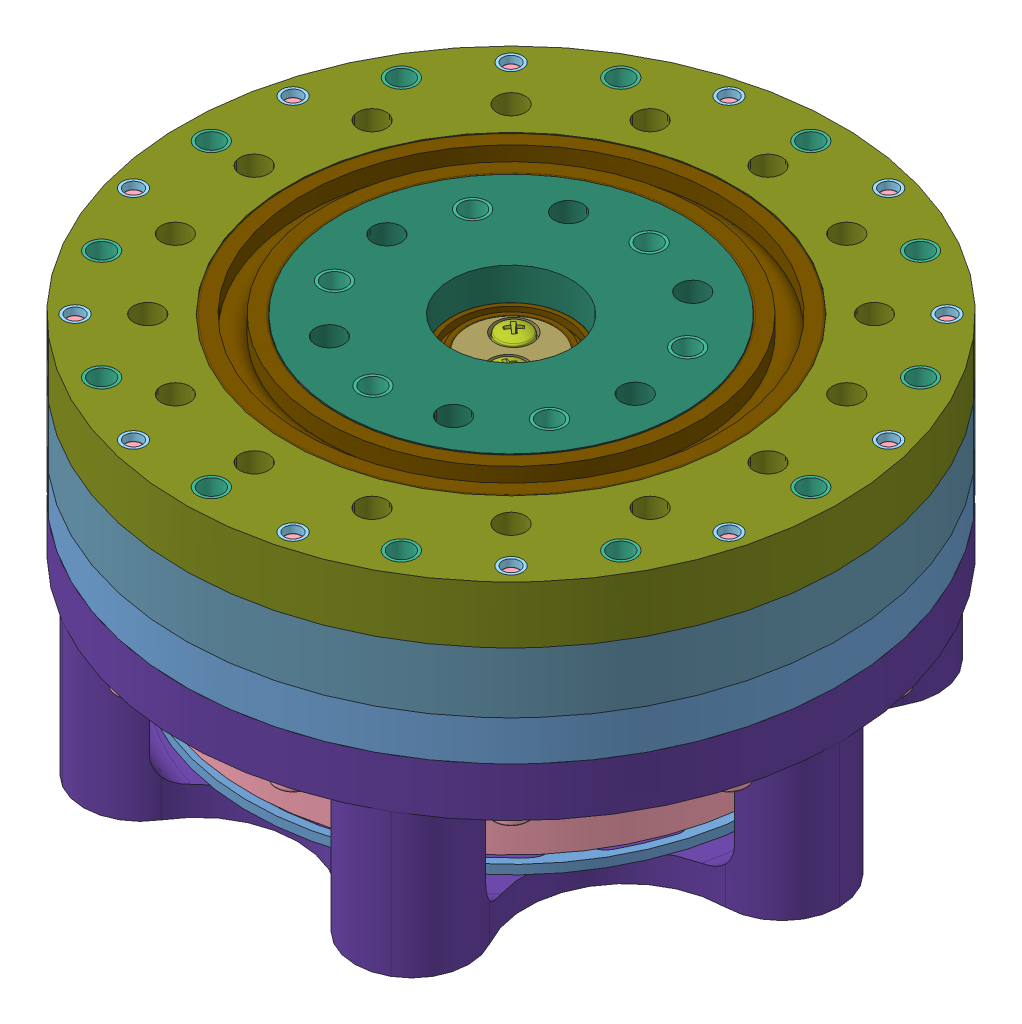
SolidWorks assembly Cycloidal, configuration Default. Lengths in mm.
Overall size (162.63 70.39 162.63).
392 component instances, 94 part files, 246 mates.
Components (placement in the parent):
- motor-X83008S.stp-1: motor-X83008S.stp [Default] at (19.7719 89.7915 55.1095) x (0.817868 0 0.575406) z (0 -1 0) size (114.7 114.7 37.62)
  - base.stp-1: base.stp [Default] at (42.0794 12.0269 46.7342) size (91.6 91.6 15.61)
  - stator.stp-1: stator.stp [Default] at (42.0794 12.0269 33.1342) x (0.08493 -0.996387 0) z (0 0 1) size (83 83 8)
  - coil.stp-1: coil.stp [Default] at (39.5332 41.8984 37.1342) x (0.996387 0.08493 0) z (-0.08493 0.996387 0) size (4.4 10.2 10.5)
  - coil.stp-2: coil.stp [Default] at (34.3848 41.0025 37.1342) x (0.966502 0.256661 0) z (-0.256661 0.966502 0) size (4.4 10.2 10.5)
  - coil.stp-3: coil.stp [Default] at (29.4701 39.2261 37.1342) x (0.90725 0.420593 0) z (-0.420593 0.90725 0) size (4.4 10.2 10.5)
  - coil.stp-4: coil.stp [Default] at (24.9386 36.6233 37.1342) x (0.820431 0.571745 0) z (-0.571745 0.820431 0) size (4.4 10.2 10.5)
  - coil.stp-5: coil.stp [Default] at (20.9279 33.2732 37.1342) x (0.708685 0.705525 0) z (-0.705525 0.708685 0) size (4.4 10.2 10.5)
  - coil.stp-6: coil.stp [Default] at (17.5599 29.2775 37.1342) x (0.575405 0.817869 0) z (-0.817869 0.575405 0) size (4.4 10.2 10.5)
  - coil.stp-7: coil.stp [Default] at (14.9368 24.7576 37.1342) x (0.424642 0.905361 0) z (-0.905361 0.424642 0) size (4.4 10.2 10.5)
  - coil.stp-8: coil.stp [Default] at (13.1385 19.8509 37.1342) x (0.260976 0.965345 0) z (-0.965345 0.260976 0) size (4.4 10.2 10.5)
  - coil.stp-9: coil.stp [Default] at (12.2196 14.7066 37.1342) x (0.089381 0.995998 0) z (-0.995998 0.089381 0) size (4.4 10.2 10.5)
  - coil.stp-10: coil.stp [Default] at (12.2079 9.4807 37.1342) x (-0.08493 0.996387 0) z (-0.996387 -0.08493 0) size (4.4 10.2 10.5)
  - coil.stp-11: coil.stp [Default] at (13.1039 4.3323 37.1342) x (-0.256661 0.966502 0) z (-0.966502 -0.256661 0) size (4.4 10.2 10.5)
  - coil.stp-12: coil.stp [Default] at (14.8802 -0.5824 37.1342) x (-0.420593 0.90725 0) z (-0.90725 -0.420593 0) size (4.4 10.2 10.5)
  - coil.stp-13: coil.stp [Default] at (17.483 -5.1139 37.1342) x (-0.571745 0.820431 0) z (-0.820431 -0.571745 0) size (4.4 10.2 10.5)
  - coil.stp-14: coil.stp [Default] at (20.8332 -9.1246 37.1342) x (-0.705525 0.708685 0) z (-0.708685 -0.705525 0) size (4.4 10.2 10.5)
  - coil.stp-15: coil.stp [Default] at (24.8289 -12.4926 37.1342) x (-0.817869 0.575405 0) z (-0.575405 -0.817869 0) size (4.4 10.2 10.5)
  - coil.stp-16: coil.stp [Default] at (29.3487 -15.1157 37.1342) x (-0.905361 0.424642 0) z (-0.424642 -0.905361 0) size (4.4 10.2 10.5)
  - coil.stp-17: coil.stp [Default] at (34.2554 -16.914 37.1342) x (-0.965345 0.260976 0) z (-0.260976 -0.965345 0) size (4.4 10.2 10.5)
  - coil.stp-18: coil.stp [Default] at (39.3998 -17.8329 37.1342) x (-0.995998 0.089381 0) z (-0.089381 -0.995998 0) size (4.4 10.2 10.5)
  - coil.stp-19: coil.stp [Default] at (44.6256 -17.8446 37.1342) x (-0.996387 -0.08493 0) z (0.08493 -0.996387 0) size (4.4 10.2 10.5)
  - coil.stp-20: coil.stp [Default] at (49.7741 -16.9486 37.1342) x (-0.966502 -0.256661 0) z (0.256661 -0.966502 0) size (4.4 10.2 10.5)
  - coil.stp-21: coil.stp [Default] at (54.6887 -15.1723 37.1342) x (-0.90725 -0.420593 0) z (0.420593 -0.90725 0) size (4.4 10.2 10.5)
  - coil.stp-22: coil.stp [Default] at (59.2202 -12.5695 37.1342) x (-0.820431 -0.571745 0) z (0.571745 -0.820431 0) size (4.4 10.2 10.5)
  - coil.stp-23: coil.stp [Default] at (63.2309 -9.2193 37.1342) x (-0.708685 -0.705525 0) z (0.705525 -0.708685 0) size (4.4 10.2 10.5)
  - coil.stp-24: coil.stp [Default] at (66.599 -5.2236 37.1342) x (-0.575405 -0.817869 0) z (0.817869 -0.575405 0) size (4.4 10.2 10.5)
  - coil.stp-25: coil.stp [Default] at (69.222 -0.7038 37.1342) x (-0.424642 -0.905361 0) z (0.905361 -0.424642 0) size (4.4 10.2 10.5)
  - coil.stp-26: coil.stp [Default] at (71.0203 4.2029 37.1342) x (-0.260976 -0.965345 0) z (0.965345 -0.260976 0) size (4.4 10.2 10.5)
  - coil.stp-27: coil.stp [Default] at (71.9392 9.3473 37.1342) x (-0.089381 -0.995998 0) z (0.995998 -0.089381 0) size (4.4 10.2 10.5)
  - coil.stp-28: coil.stp [Default] at (71.9509 14.5731 37.1342) x (0.08493 -0.996387 0) z (0.996387 0.08493 0) size (4.4 10.2 10.5)
  - coil.stp-29: coil.stp [Default] at (71.055 19.7216 37.1342) x (0.256661 -0.966502 0) z (0.966502 0.256661 0) size (4.4 10.2 10.5)
  - coil.stp-30: coil.stp [Default] at (69.2786 24.6362 37.1342) x (0.420593 -0.90725 0) z (0.90725 0.420593 0) size (4.4 10.2 10.5)
  - coil.stp-31: coil.stp [Default] at (66.6758 29.1677 37.1342) x (0.571745 -0.820431 0) z (0.820431 0.571745 0) size (4.4 10.2 10.5)
  - coil.stp-32: coil.stp [Default] at (63.3257 33.1785 37.1342) x (0.705525 -0.708685 0) z (0.708685 0.705525 0) size (4.4 10.2 10.5)
  - coil.stp-33: coil.stp [Default] at (59.33 36.5465 37.1342) x (0.817869 -0.575405 0) z (0.575405 0.817869 0) size (4.4 10.2 10.5)
  - coil.stp-34: coil.stp [Default] at (54.8101 39.1695 37.1342) x (0.905361 -0.424642 0) z (0.424642 0.905361 0) size (4.4 10.2 10.5)
  - coil.stp-35: coil.stp [Default] at (49.9034 40.9678 37.1342) x (0.965345 -0.260976 0) z (0.260976 0.965345 0) size (4.4 10.2 10.5)
  - coil.stp-36: coil.stp [Default] at (44.759 41.8868 37.1342) x (0.995998 -0.089381 0) z (0.089381 0.995998 0) size (4.4 10.2 10.5)
  - rotor.stp-1: rotor.stp [Default] at (42.0794 12.0269 42.1342) x (-0.293442 0.955977 0) z (0 0 -1) size (91.8 91.8 12)
  - outrunner.stp-1: outrunner.stp [Default] at (42.0794 12.0269 30.1342) x (-0.254711 0.967017 0) z (-0.967017 -0.254711 0) size (91.8 17.01 91.8)
  - screw-mount.stp-1: screw-mount.stp [Default] at (38.1314 27.0157 27.1342) x (1 0 0) z (0 0 -1) size (7 7 6.5)
  - screw-mount.stp-2: screw-mount.stp [Default] at (27.0906 8.0789 27.1342) x (1 0 0) z (0 0 -1) size (7 7 6.5)
  - screw-mount.stp-3: screw-mount.stp [Default] at (57.0682 15.9749 27.1342) x (1 0 0) z (0 0 -1) size (7 7 6.5)
  - screw-mount.stp-4: screw-mount.stp [Default] at (46.0274 -2.9618 27.1342) x (1 0 0) z (0 0 -1) size (7 7 6.5)
  - 6702ZZ-bearing-15x21x4.stp-1: 6702ZZ-bearing-15x21x4.stp [Default] at (42.0794 12.0269 43.7342) x (1 0 0) z (0 -1 0) size (21 4 21)
  - 6702ZZ-bearing-15x21x4.stp-2: 6702ZZ-bearing-15x21x4.stp [Default] at (42.0794 12.0269 35.1342) x (1 0 0) z (0 1 0) size (21 4 21)
  - shaft.stp-1: shaft.stp [Default] at (42.0794 12.0269 20.1342) size (16 16 31.6)
  - fix-screw.stp-1: fix-screw.stp [Default] at (42.0794 12.0269 51.7342) x (1 0 0) z (0 0 -1) size (19.67 18.96 12.02)
- Base_Plate-1: Base_Plate [Default] at (47.267 69.6573 89.1587) x (-0.64433 0 -0.764747) z (0.764747 0 -0.64433) size (40 7 40)
- Eccentric_Shaft-1: Eccentric_Shaft [Default] at (62.181 70.3165 95.0179) x (-0.764747 0 0.64433) z (-0.64433 0 -0.764747) size (20 15 17)
  - Eccentric_Shaft_bot-1: Eccentric_Shaft_bot [Default] at (7.6302 6.3409 14.0904) size (17 5 17)
  - Eccentric_Shaft_bot-2: Eccentric_Shaft_bot [Default] at (7.6302 11.3409 14.0904) x (-1 0 0) z (0 0 -1) size (17 5 17)
  - Eccentric_Shaft_top-1: Eccentric_Shaft_top [Default] at (7.6302 16.3409 14.0904) x (-1 0 0) z (0 0 -1) size (17 5 17)
- Cycloidal_Discs-1: Cycloidal_Discs [Default] at (46.1199 86.6573 90.1252) x (0.999784 0 -0.020763) z (-0.020763 0 -0.999784) size (79.25 5 79.73)
- Cycloidal_Discs-2: Cycloidal_Discs [Default] at (48.4141 76.6573 88.1922) x (0.979859 0 0.19969) z (-0.19969 0 0.979859) size (79.25 5 79.73)
- Ring_Pin_Housing-1: Ring_Pin_Housing [Default] at (47.267 76.6573 89.1587) x (0.707107 0 -0.707107) z (0.707107 0 0.707107) size (115 10.6 115)
- Output_Shaft-1: Output_Shaft [Default] at (47.267 87.2573 89.1587) x (-0.998587 0 -0.053142) z (0.053142 0 -0.998587) size (60 10 60)
- Cover-1: Cover [Default] at (47.267 87.2573 89.1587) x (0.707107 0 -0.707107) z (0.707107 0 0.707107) size (115 10.4 115)
- Motor_Cover-2: Motor_Cover [Default] at (47.267 36.0573 89.1587) size (115 33.6 115)
- radial ball bearing_68_iso-39: radial ball bearing_68_iso [ISO 15 RBB - 1860 - 32,SI,NC,32_68] at (47.267 92.2573 89.1587) x (0 1 0) z (0 0 1) size (10 78 78)
- radial ball bearing_68_iso-40: radial ball bearing_68_iso [ISO 15 RBB - 1840 - 32,SI,NC,32_68] at (47.267 72.9573 89.1587) x (0 1 0) z (0.001003 0 0.999999) size (7 52 52)
- Base_plate_2-1: Base_plate_2 [Default] at (47.267 69.6573 89.1587) x (0.707107 0 -0.707107) z (0.707107 0 0.707107) size (115 7 115)
- m13_bearing-31: m13_bearing [Default] at (-10.7414 95.4081 67.0593) x (0.227678 0 0.973736) z (0.973736 0 -0.227678) size (13 16 13)
  - m6-1: m6 [Default] at (8.4921 2.5508 14.8914) size (6 16 6)
  - radial ball bearing_68_iso-1: radial ball bearing_68_iso [ISO 15 RBB - 286 - 10,SI,NC,10_68] at (8.4921 16.0508 14.8914) x (0 1 0) z (0 0 1) size (5 13 13)
  - radial ball bearing_68_iso-2: radial ball bearing_68_iso [ISO 15 RBB - 286 - 10,SI,NC,10_68] at (8.4921 11.0508 14.8914) x (0 1 0) z (0 0 1) size (5 13 13)
- m13_bearing-32: m13_bearing [Default] at (-14.1668 95.4081 84.2801) x (0.227678 0 0.973736) z (0.973736 0 -0.227678) size (13 16 13)
  - m6-1: m6 [Default] at (8.4921 2.5508 14.8914) size (6 16 6)
  - radial ball bearing_68_iso-1: radial ball bearing_68_iso [ISO 15 RBB - 286 - 10,SI,NC,10_68] at (8.4921 16.0508 14.8914) x (0 1 0) z (0 0 1) size (5 13 13)
  - radial ball bearing_68_iso-2: radial ball bearing_68_iso [ISO 15 RBB - 286 - 10,SI,NC,10_68] at (8.4921 11.0508 14.8914) x (0 1 0) z (0 0 1) size (5 13 13)
- m13_bearing-34: m13_bearing [Default] at (13.6125 95.5581 125.8547) x (0.227678 0 0.973736) z (0.973736 0 -0.227678) size (13 16 13)
  - m6-1: m6 [Default] at (8.4921 2.5508 14.8914) size (6 16 6)
  - radial ball bearing_68_iso-1: radial ball bearing_68_iso [ISO 15 RBB - 286 - 10,SI,NC,10_68] at (8.4921 16.0508 14.8914) x (0 1 0) z (0 0 1) size (5 13 13)
  - radial ball bearing_68_iso-2: radial ball bearing_68_iso [ISO 15 RBB - 286 - 10,SI,NC,10_68] at (8.4921 11.0508 14.8914) x (0 1 0) z (0 0 1) size (5 13 13)
- m13_bearing-35: m13_bearing [Default] at (-0.9866 95.4081 116.0999) x (0.227678 0 0.973736) z (0.973736 0 -0.227678) size (13 16 13)
  - m6-1: m6 [Default] at (8.4921 2.5508 14.8914) size (6 16 6)
  - radial ball bearing_68_iso-1: radial ball bearing_68_iso [ISO 15 RBB - 286 - 10,SI,NC,10_68] at (8.4921 16.0508 14.8914) x (0 1 0) z (0 0 1) size (5 13 13)
  - radial ball bearing_68_iso-2: radial ball bearing_68_iso [ISO 15 RBB - 286 - 10,SI,NC,10_68] at (8.4921 11.0508 14.8914) x (0 1 0) z (0 0 1) size (5 13 13)
- m13_bearing-36: m13_bearing [Default] at (-10.7414 95.5581 101.5009) x (0.227678 0 0.973736) z (0.973736 0 -0.227678) size (13 16 13)
  - m6-1: m6 [Default] at (8.4921 2.5508 14.8914) size (6 16 6)
  - radial ball bearing_68_iso-1: radial ball bearing_68_iso [ISO 15 RBB - 286 - 10,SI,NC,10_68] at (8.4921 16.0508 14.8914) x (0 1 0) z (0 0 1) size (5 13 13)
  - radial ball bearing_68_iso-2: radial ball bearing_68_iso [ISO 15 RBB - 286 - 10,SI,NC,10_68] at (8.4921 11.0508 14.8914) x (0 1 0) z (0 0 1) size (5 13 13)
- m13_bearing-1: m13_bearing [Default] at (-0.8801 95.4081 62.5627) x (0.736525 0 0.676411) z (0.676411 0 -0.736525) size (13 16 13)
  - m6-1: m6 [Default] at (8.4921 2.5508 14.8914) size (6 16 6)
  - radial ball bearing_68_iso-1: radial ball bearing_68_iso [ISO 15 RBB - 286 - 10,SI,NC,10_68] at (8.4921 16.0508 14.8914) x (0 1 0) z (0 0 1) size (5 13 13)
  - radial ball bearing_68_iso-2: radial ball bearing_68_iso [ISO 15 RBB - 286 - 10,SI,NC,10_68] at (8.4921 11.0508 14.8914) x (0 1 0) z (0 0 1) size (5 13 13)
- m13_bearing-2: m13_bearing [Default] at (48.6831 95.4081 124.0939) x (0.120271 0 0.992741) z (0.992741 0 -0.120271) size (13 16 13)
  - m6-1: m6 [Default] at (8.4921 2.5508 14.8914) size (6 16 6)
  - radial ball bearing_68_iso-1: radial ball bearing_68_iso [ISO 15 RBB - 286 - 10,SI,NC,10_68] at (8.4921 16.0508 14.8914) x (0 1 0) z (0 0 1) size (5 13 13)
  - radial ball bearing_68_iso-2: radial ball bearing_68_iso [ISO 15 RBB - 286 - 10,SI,NC,10_68] at (8.4921 11.0508 14.8914) x (0 1 0) z (0 0 1) size (5 13 13)
- m13_bearing-3: m13_bearing [Default] at (32.7832 95.4081 34.9886) x (-0.046141 0 0.998935) z (0.998935 0 0.046141) size (13 16 13)
  - m6-1: m6 [Default] at (8.4921 2.5508 14.8914) size (6 16 6)
  - radial ball bearing_68_iso-1: radial ball bearing_68_iso [ISO 15 RBB - 286 - 10,SI,NC,10_68] at (8.4921 16.0508 14.8914) x (0 1 0) z (0 0 1) size (5 13 13)
  - radial ball bearing_68_iso-2: radial ball bearing_68_iso [ISO 15 RBB - 286 - 10,SI,NC,10_68] at (8.4921 11.0508 14.8914) x (0 1 0) z (0 0 1) size (5 13 13)
- m13_bearing-4: m13_bearing [Default] at (77.1902 95.4081 81.0003) x (0.022268 0 0.999752) z (0.999752 0 -0.022268) size (13 16 13)
  - m6-1: m6 [Default] at (8.4921 2.5508 14.8914) size (6 16 6)
  - radial ball bearing_68_iso-1: radial ball bearing_68_iso [ISO 15 RBB - 286 - 10,SI,NC,10_68] at (8.4921 16.0508 14.8914) x (0 1 0) z (0 0 1) size (5 13 13)
  - radial ball bearing_68_iso-2: radial ball bearing_68_iso [ISO 15 RBB - 286 - 10,SI,NC,10_68] at (8.4921 11.0508 14.8914) x (0 1 0) z (0 0 1) size (5 13 13)
- m13_bearing-5: m13_bearing [Default] at (73.474 95.4081 98.7828) x (0.059133 0 0.99825) z (0.99825 0 -0.059133) size (13 16 13)
  - m6-1: m6 [Default] at (8.4921 2.5508 14.8914) size (6 16 6)
  - radial ball bearing_68_iso-1: radial ball bearing_68_iso [ISO 15 RBB - 286 - 10,SI,NC,10_68] at (8.4921 16.0508 14.8914) x (0 1 0) z (0 0 1) size (5 13 13)
  - radial ball bearing_68_iso-2: radial ball bearing_68_iso [ISO 15 RBB - 286 - 10,SI,NC,10_68] at (8.4921 11.0508 14.8914) x (0 1 0) z (0 0 1) size (5 13 13)
- m13_bearing-6: m13_bearing [Default] at (12.9248 95.4081 46.7315) x (0.451561 0 0.89224) z (0.89224 0 -0.451561) size (13 16 13)
  - m6-1: m6 [Default] at (8.4921 2.5508 14.8914) size (6 16 6)
  - radial ball bearing_68_iso-1: radial ball bearing_68_iso [ISO 15 RBB - 286 - 10,SI,NC,10_68] at (8.4921 16.0508 14.8914) x (0 1 0) z (0 0 1) size (5 13 13)
  - radial ball bearing_68_iso-2: radial ball bearing_68_iso [ISO 15 RBB - 286 - 10,SI,NC,10_68] at (8.4921 11.0508 14.8914) x (0 1 0) z (0 0 1) size (5 13 13)
- m13_bearing-7: m13_bearing [Default] at (56.6452 95.4081 32.3406) x (-0.545813 0 0.837907) z (0.837907 0 0.545813) size (13 16 13)
  - m6-1: m6 [Default] at (8.4921 2.5508 14.8914) size (6 16 6)
  - radial ball bearing_68_iso-1: radial ball bearing_68_iso [ISO 15 RBB - 286 - 10,SI,NC,10_68] at (8.4921 16.0508 14.8914) x (0 1 0) z (0 0 1) size (5 13 13)
  - radial ball bearing_68_iso-2: radial ball bearing_68_iso [ISO 15 RBB - 286 - 10,SI,NC,10_68] at (8.4921 11.0508 14.8914) x (0 1 0) z (0 0 1) size (5 13 13)
- m13_bearing-8: m13_bearing [Default] at (63.0373 95.4081 51.3153) x (0.158553 0 0.98735) z (0.98735 0 -0.158553) size (13 16 13)
  - m6-1: m6 [Default] at (8.4921 2.5508 14.8914) size (6 16 6)
  - radial ball bearing_68_iso-1: radial ball bearing_68_iso [ISO 15 RBB - 286 - 10,SI,NC,10_68] at (8.4921 16.0508 14.8914) x (0 1 0) z (0 0 1) size (5 13 13)
  - radial ball bearing_68_iso-2: radial ball bearing_68_iso [ISO 15 RBB - 286 - 10,SI,NC,10_68] at (8.4921 11.0508 14.8914) x (0 1 0) z (0 0 1) size (5 13 13)
- m13_bearing-9: m13_bearing [Default] at (83.8577 95.4081 55.5358) x (-0.687134 0 0.72653) z (0.72653 0 0.687134) size (13 16 13)
  - m6-1: m6 [Default] at (8.4921 2.5508 14.8914) size (6 16 6)
  - radial ball bearing_68_iso-1: radial ball bearing_68_iso [ISO 15 RBB - 286 - 10,SI,NC,10_68] at (8.4921 16.0508 14.8914) x (0 1 0) z (0 0 1) size (5 13 13)
  - radial ball bearing_68_iso-2: radial ball bearing_68_iso [ISO 15 RBB - 286 - 10,SI,NC,10_68] at (8.4921 11.0508 14.8914) x (0 1 0) z (0 0 1) size (5 13 13)
- m13_bearing-11: m13_bearing [Default] at (30.1977 95.4081 135.7424) x (0.57351 0 0.819198) z (0.819198 0 -0.57351) size (13 16 13)
  - m6-1: m6 [Default] at (8.4921 2.5508 14.8914) size (6 16 6)
  - radial ball bearing_68_iso-1: radial ball bearing_68_iso [ISO 15 RBB - 286 - 10,SI,NC,10_68] at (8.4921 16.0508 14.8914) x (0 1 0) z (0 0 1) size (5 13 13)
  - radial ball bearing_68_iso-2: radial ball bearing_68_iso [ISO 15 RBB - 286 - 10,SI,NC,10_68] at (8.4921 11.0508 14.8914) x (0 1 0) z (0 0 1) size (5 13 13)
- m13_bearing-12: m13_bearing [Default] at (62.8861 95.4081 115.3744) x (0.184178 0 0.982893) z (0.982893 0 -0.184178) size (13 16 13)
  - m6-1: m6 [Default] at (8.4921 2.5508 14.8914) size (6 16 6)
  - radial ball bearing_68_iso-1: radial ball bearing_68_iso [ISO 15 RBB - 286 - 10,SI,NC,10_68] at (8.4921 16.0508 14.8914) x (0 1 0) z (0 0 1) size (5 13 13)
  - radial ball bearing_68_iso-2: radial ball bearing_68_iso [ISO 15 RBB - 286 - 10,SI,NC,10_68] at (8.4921 11.0508 14.8914) x (0 1 0) z (0 0 1) size (5 13 13)
- socket button head screw_iso-2: socket button head screw_iso [ISO 7380 - M4 x 12 - 12N] at (47.267 67.4573 134.1587) x (0 1 0) z (-0.724148 0 0.689645) size (14.2 7.6 7.6)
- socket button head screw_iso-3: socket button head screw_iso [ISO 7380 - M4 x 12 - 12N] at (15.4472 67.4573 57.3389) x (0 1 0) z (-0.724148 0 0.689645) size (14.2 7.6 7.6)
- socket button head screw_iso-4: socket button head screw_iso [ISO 7380 - M4 x 12 - 12N] at (30.0462 67.4573 47.5841) x (0 1 0) z (-0.724148 0 0.689645) size (14.2 7.6 7.6)
- socket button head screw_iso-5: socket button head screw_iso [ISO 7380 - M4 x 12 - 12N] at (47.267 67.4573 44.1587) x (0 1 0) z (-0.724148 0 0.689645) size (14.2 7.6 7.6)
- socket button head screw_iso-6: socket button head screw_iso [ISO 7380 - M4 x 12 - 12N] at (64.4877 67.4573 47.5841) x (0 1 0) z (-0.724148 0 0.689645) size (14.2 7.6 7.6)
- socket button head screw_iso-8: socket button head screw_iso [ISO 7380 - M4 x 12 - 12N] at (88.8416 67.4573 71.9379) x (0 1 0) z (-0.724148 0 0.689645) size (14.2 7.6 7.6)
- socket button head screw_iso-9: socket button head screw_iso [ISO 7380 - M4 x 12 - 12N] at (92.267 67.4573 89.1587) x (0 1 0) z (-0.724148 0 0.689645) size (14.2 7.6 7.6)
- socket button head screw_iso-10: socket button head screw_iso [ISO 7380 - M4 x 12 - 12N] at (88.8416 67.4573 106.3794) x (0 1 0) z (-0.724148 0 0.689645) size (14.2 7.6 7.6)
- socket button head screw_iso-11: socket button head screw_iso [ISO 7380 - M4 x 12 - 12N] at (79.0868 67.4573 120.9785) x (0 1 0) z (-0.724148 0 0.689645) size (14.2 7.6 7.6)
- M3x35-6: M3x35 [Default] at (9.0832 59.8573 50.9749) size (6 36.2 6)
- M3x35-7: M3x35 [Default] at (-4.893 59.8573 75.1824) size (6 36.2 6)
- M3x35-8: M3x35 [Default] at (-4.893 59.8573 103.1349) size (6 36.2 6)
- M3x35-9: M3x35 [Default] at (9.0832 59.8573 127.3424) size (6 36.2 6)
- M3x35-10: M3x35 [Default] at (33.2908 59.8573 141.3187) size (6 36.2 6)
- M3x35-11: M3x35 [Default] at (61.2432 59.8573 141.3187) size (6 36.2 6)
- M3x35-12: M3x35 [Default] at (85.4508 59.8573 127.3424) size (6 36.2 6)
- M3x35-13: M3x35 [Default] at (99.427 59.8573 103.1349) size (6 36.2 6)
- M3x35-14: M3x35 [Default] at (99.427 59.8573 75.1824) size (6 36.2 6)
- M3x35-15: M3x35 [Default] at (85.4508 59.8573 50.9749) size (6 36.2 6)
- M3x35-16: M3x35 [Default] at (33.2908 59.8573 36.9987) size (6 36.2 6)
- M3x35-17: M3x35 [Default] at (61.2432 59.8573 36.9987) size (6 36.2 6)
- m13_bearing-13: m13_bearing [Default] at (21.9503 95.0081 60.165) x (0 0 1) z (1 0 0) size (13 16 13)
  - m6-1: m6 [Default] at (8.4921 2.5508 14.8914) size (6 16 6)
  - radial ball bearing_68_iso-1: radial ball bearing_68_iso [ISO 15 RBB - 286 - 10,SI,NC,10_68] at (8.4921 16.0508 14.8914) x (0 1 0) z (0 0 1) size (5 13 13)
  - radial ball bearing_68_iso-2: radial ball bearing_68_iso [ISO 15 RBB - 286 - 10,SI,NC,10_68] at (8.4921 11.0508 14.8914) x (0 1 0) z (0 0 1) size (5 13 13)
- m13_bearing-14: m13_bearing [Default] at (31.351 95.0081 72.3113) x (-0.995553 0 0.094199) z (0.094199 0 0.995553) size (13 16 13)
  - m6-1: m6 [Default] at (8.4921 2.5508 14.8914) size (6 16 6)
  - radial ball bearing_68_iso-1: radial ball bearing_68_iso [ISO 15 RBB - 286 - 10,SI,NC,10_68] at (8.4921 16.0508 14.8914) x (0 1 0) z (0 0 1) size (5 13 13)
  - radial ball bearing_68_iso-2: radial ball bearing_68_iso [ISO 15 RBB - 286 - 10,SI,NC,10_68] at (8.4921 11.0508 14.8914) x (0 1 0) z (0 0 1) size (5 13 13)
- m13_bearing-15: m13_bearing [Default] at (19.8333 95.0081 99.9459) x (0 0 1) z (1 0 0) size (13 16 13)
  - m6-1: m6 [Default] at (8.4921 2.5508 14.8914) size (6 16 6)
  - radial ball bearing_68_iso-1: radial ball bearing_68_iso [ISO 15 RBB - 286 - 10,SI,NC,10_68] at (8.4921 16.0508 14.8914) x (0 1 0) z (0 0 1) size (5 13 13)
  - radial ball bearing_68_iso-2: radial ball bearing_68_iso [ISO 15 RBB - 286 - 10,SI,NC,10_68] at (8.4921 11.0508 14.8914) x (0 1 0) z (0 0 1) size (5 13 13)
- m13_bearing-16: m13_bearing [Default] at (60.3496 95.0081 87.0135) x (0.852631 0 -0.522513) z (-0.522513 0 -0.852631) size (13 16 13)
  - m6-1: m6 [Default] at (8.4921 2.5508 14.8914) size (6 16 6)
  - radial ball bearing_68_iso-1: radial ball bearing_68_iso [ISO 15 RBB - 286 - 10,SI,NC,10_68] at (8.4921 16.0508 14.8914) x (0 1 0) z (0 0 1) size (5 13 13)
  - radial ball bearing_68_iso-2: radial ball bearing_68_iso [ISO 15 RBB - 286 - 10,SI,NC,10_68] at (8.4921 11.0508 14.8914) x (0 1 0) z (0 0 1) size (5 13 13)
- m13_bearing-17: m13_bearing [Default] at (45.2305 95.0081 121.432) x (0.95663 0 0.291306) z (0.291306 0 -0.95663) size (13 16 13)
  - m6-1: m6 [Default] at (8.4921 2.5508 14.8914) size (6 16 6)
  - radial ball bearing_68_iso-1: radial ball bearing_68_iso [ISO 15 RBB - 286 - 10,SI,NC,10_68] at (8.4921 16.0508 14.8914) x (0 1 0) z (0 0 1) size (5 13 13)
  - radial ball bearing_68_iso-2: radial ball bearing_68_iso [ISO 15 RBB - 286 - 10,SI,NC,10_68] at (8.4921 11.0508 14.8914) x (0 1 0) z (0 0 1) size (5 13 13)
- m13_bearing-18: m13_bearing [Default] at (55.3431 95.0081 81.8889) x (0 0 1) z (1 0 0) size (13 16 13)
  - m6-1: m6 [Default] at (8.4921 2.5508 14.8914) size (6 16 6)
  - radial ball bearing_68_iso-1: radial ball bearing_68_iso [ISO 15 RBB - 286 - 10,SI,NC,10_68] at (8.4921 16.0508 14.8914) x (0 1 0) z (0 0 1) size (5 13 13)
  - radial ball bearing_68_iso-2: radial ball bearing_68_iso [ISO 15 RBB - 286 - 10,SI,NC,10_68] at (8.4921 11.0508 14.8914) x (0 1 0) z (0 0 1) size (5 13 13)
- M3x4x4.2_brass_insert-1: M3x4x4.2_brass_insert [Default] at (-4.893 93.2573 75.1824) x (0.984609 0 -0.174769) z (0.174769 0 0.984609) size (4 4 4)
- M3x4x4.2_brass_insert-2: M3x4x4.2_brass_insert [Default] at (9.0832 97.2573 50.9749) x (-0.680278 0 -0.732954) z (-0.732954 0 0.680278) size (4 4 4)
- M3x4x4.2_brass_insert-3: M3x4x4.2_brass_insert [Default] at (33.2908 97.2573 36.9987) x (-0.509546 0 -0.860444) z (-0.860444 0 0.509546) size (4 4 4)
- M3x4x4.2_brass_insert-6: M3x4x4.2_brass_insert [Default] at (99.427 97.2573 75.1824) x (-0.680278 0 -0.732954) z (-0.732954 0 0.680278) size (4 4 4)
- M3x4x4.2_brass_insert-8: M3x4x4.2_brass_insert [Default] at (85.4508 93.2573 127.3424) x (-0.970393 0 0.241533) z (-0.241533 0 -0.970393) size (4 4 4)
- M3x4x4.2_brass_insert-14: M3x4x4.2_brass_insert [Default] at (61.2432 97.2573 36.9987) x (0.509546 0 0.860444) z (0.860444 0 -0.509546) size (4 4 4)
- M3x4x4.2_brass_insert-15: M3x4x4.2_brass_insert [Default] at (85.4508 93.2573 50.9749) x (0.897191 0 -0.441644) z (0.441644 0 0.897191) size (4 4 4)
- M3x4x4.2_brass_insert-16: M3x4x4.2_brass_insert [Default] at (99.427 97.2573 103.1349) x (-0.680278 0 -0.732954) z (-0.732954 0 0.680278) size (4 4 4)
- M3x4x4.2_brass_insert-17: M3x4x4.2_brass_insert [Default] at (61.2432 97.2573 141.3187) x (0.680278 0 0.732954) z (0.732954 0 -0.680278) size (4 4 4)
- M3x4x4.2_brass_insert-19: M3x4x4.2_brass_insert [Default] at (33.2908 97.2573 141.3187) x (0.680278 0 0.732954) z (0.732954 0 -0.680278) size (4 4 4)
- M3x4x4.2_brass_insert-20: M3x4x4.2_brass_insert [Default] at (9.0832 97.2573 127.3424) x (0.680278 0 0.732954) z (0.732954 0 -0.680278) size (4 4 4)
- M3x4x4.2_brass_insert-21: M3x4x4.2_brass_insert [Default] at (-4.893 97.2573 103.1349) x (0.680278 0 0.732954) z (0.732954 0 -0.680278) size (4 4 4)
- M4x6x5.5_brass_insert-47: M4x6x5.5_brass_insert [Default] at (5.6924 92.8573 71.9379) x (0.474598 0 0.880203) z (0 1 0) size (5 5 6)
- M4x6x5.5_brass_insert-48: M4x6x5.5_brass_insert [Default] at (2.267 92.8573 89.1587) x (0.260051 0 0.965595) z (0 1 0) size (5 5 6)
- M4x6x5.5_brass_insert-49: M4x6x5.5_brass_insert [Default] at (5.6924 87.0073 106.3794) x (-0.745833 0 0.666133) z (0 -1 0) size (5 5 6)
- M4x6x5.5_brass_insert-50: M4x6x5.5_brass_insert [Default] at (15.4472 86.8573 120.9785) x (-0.745833 0 0.666133) z (0 -1 0) size (5 5 6)
- M4x6x5.5_brass_insert-51: M4x6x5.5_brass_insert [Default] at (30.0462 87.0073 130.7332) x (0.260051 0 -0.965595) z (0 -1 0) size (5 5 6)
- M4x6x5.5_brass_insert-1: M4x6x5.5_brass_insert [Default] at (36.8417 86.4573 68.6571) x (-0.745833 0 0.666133) z (0 -1 0) size (5 5 6)
- M4x6x5.5_brass_insert-4: M4x6x5.5_brass_insert [Default] at (70.2345 92.4573 90.3809) x (0.260051 0 0.965595) z (0 1 0) size (5 5 6)
- M4x6x5.5_brass_insert-5: M4x6x5.5_brass_insert [Default] at (57.6922 92.4573 109.6602) x (0.260051 0 0.965595) z (0 1 0) size (5 5 6)
- M4x6x5.5_brass_insert-6: M4x6x5.5_brass_insert [Default] at (34.7247 92.4573 108.438) x (0.260051 0 0.965595) z (0 1 0) size (5 5 6)
- M4x6x5.5_brass_insert-7: M4x6x5.5_brass_insert [Default] at (24.2995 92.4573 87.9364) x (0.175665 0 0.98445) z (0 1 0) size (5 5 6)
- M4x6x5.5_brass_insert-8: M4x6x5.5_brass_insert [Default] at (48.4892 97.2573 66.1912) x (0.260051 0 0.965595) z (0 1 0) size (5 5 6)
- M4x6x5.5_brass_insert-9: M4x6x5.5_brass_insert [Default] at (27.9877 97.2573 76.6164) x (0.260051 0 0.965595) z (0 1 0) size (5 5 6)
- M4x6x5.5_brass_insert-10: M4x6x5.5_brass_insert [Default] at (26.7654 97.2573 99.5839) x (0.260051 0 0.965595) z (0 1 0) size (5 5 6)
- M4x6x5.5_brass_insert-11: M4x6x5.5_brass_insert [Default] at (46.0447 97.2573 112.1262) x (0.260051 0 0.965595) z (0 1 0) size (5 5 6)
- M4x6x5.5_brass_insert-13: M4x6x5.5_brass_insert [Default] at (66.5463 97.2573 101.7009) x (0.260051 0 0.965595) z (0 1 0) size (5 5 6)
- M4x6x5.5_brass_insert-14: M4x6x5.5_brass_insert [Default] at (67.7686 97.2573 78.7334) x (0.260051 0 0.965595) z (0 1 0) size (5 5 6)
- M4x6x5.5_brass_insert-15: M4x6x5.5_brass_insert [Default] at (59.8092 92.4573 69.8794) x (0.151918 0 0.988393) z (0 1 0) size (5 5 6)
- M4x6x5.5_brass_insert-20: M4x6x5.5_brass_insert [Default] at (64.4877 86.8573 130.7332) x (-0.745833 0 0.666133) z (0 -1 0) size (5 5 6)
- M4x6x5.5_brass_insert-21: M4x6x5.5_brass_insert [Default] at (47.267 86.8573 134.1587) x (-0.745833 0 0.666133) z (0 -1 0) size (5 5 6)
- M4x6x5.5_brass_insert-22: M4x6x5.5_brass_insert [Default] at (15.4472 86.8573 57.3389) x (0.623293 0 0.781988) z (0 -1 0) size (5 5 6)
- M4x6x5.5_brass_insert-23: M4x6x5.5_brass_insert [Default] at (30.0462 86.8573 47.5841) x (0.623293 0 0.781988) z (0 -1 0) size (5 5 6)
- M4x6x5.5_brass_insert-24: M4x6x5.5_brass_insert [Default] at (79.0868 86.8573 120.9785) x (0.541965 0 0.840401) z (0 -1 0) size (5 5 6)
- M4x6x5.5_brass_insert-25: M4x6x5.5_brass_insert [Default] at (88.8416 86.8573 106.3794) x (-0.745833 0 0.666133) z (0 -1 0) size (5 5 6)
- M4x6x5.5_brass_insert-26: M4x6x5.5_brass_insert [Default] at (92.267 86.8573 89.1587) x (-0.745833 0 0.666133) z (0 -1 0) size (5 5 6)
- M4x6x5.5_brass_insert-27: M4x6x5.5_brass_insert [Default] at (88.8416 86.8573 71.9379) x (-0.745833 0 0.666133) z (0 -1 0) size (5 5 6)
- M4x6x5.5_brass_insert-28: M4x6x5.5_brass_insert [Default] at (79.0868 92.8573 57.3389) x (0.260051 0 0.965595) z (0 1 0) size (5 5 6)
- M4x6x5.5_brass_insert-29: M4x6x5.5_brass_insert [Default] at (64.4877 86.8573 47.5841) x (-0.142939 0 0.989731) z (0 -1 0) size (5 5 6)
- M4x6x5.5_brass_insert-31: M4x6x5.5_brass_insert [Default] at (47.267 86.8573 44.1587) x (-0.220341 0 0.975423) z (0 -1 0) size (5 5 6)
- M4x6x5.5_brass_insert-34: M4x6x5.5_brass_insert [Default] at (1.8007 97.2573 62.9087) x (0.260051 0 0.965595) z (0 1 0) size (5 5 6)
- M4x6x5.5_brass_insert-35: M4x6x5.5_brass_insert [Default] at (-5.233 97.2573 89.1587) x (0.260051 0 0.965595) z (0 1 0) size (5 5 6)
- M4x6x5.5_brass_insert-36: M4x6x5.5_brass_insert [Default] at (1.8007 97.2573 115.4087) x (0.260051 0 0.965595) z (0 1 0) size (5 5 6)
- M4x6x5.5_brass_insert-37: M4x6x5.5_brass_insert [Default] at (21.017 97.2573 134.625) x (0.260051 0 0.965595) z (0 1 0) size (5 5 6)
- M4x6x5.5_brass_insert-38: M4x6x5.5_brass_insert [Default] at (47.267 97.2573 141.6587) x (0.260051 0 0.965595) z (0 1 0) size (5 5 6)
- M4x6x5.5_brass_insert-39: M4x6x5.5_brass_insert [Default] at (73.517 97.2573 134.625) x (0.260051 0 0.965595) z (0 1 0) size (5 5 6)
- M4x6x5.5_brass_insert-40: M4x6x5.5_brass_insert [Default] at (92.7333 97.2573 115.4087) x (0.260051 0 0.965595) z (0 1 0) size (5 5 6)
- M4x6x5.5_brass_insert-41: M4x6x5.5_brass_insert [Default] at (99.767 97.2573 89.1587) x (0.260051 0 0.965595) z (0 1 0) size (5 5 6)
- M4x6x5.5_brass_insert-42: M4x6x5.5_brass_insert [Default] at (92.7333 97.2573 62.9087) x (0.260051 0 0.965595) z (0 1 0) size (5 5 6)
- M4x6x5.5_brass_insert-43: M4x6x5.5_brass_insert [Default] at (73.517 97.2573 43.6923) x (0.260051 0 0.965595) z (0 1 0) size (5 5 6)
- M4x6x5.5_brass_insert-44: M4x6x5.5_brass_insert [Default] at (47.267 97.2573 36.6587) x (0.260051 0 0.965595) z (0 1 0) size (5 5 6)
- M4x6x5.5_brass_insert-45: M4x6x5.5_brass_insert [Default] at (21.017 97.2573 43.6923) x (0.260051 0 0.965595) z (0 1 0) size (5 5 6)
- pan cross head_am-1: pan cross head_am [B18.6.7M - M3 x 0.5 x 20 Type I Cross Recessed PHMS --20N] at (44.6897 92.5573 86.0997) x (0 -1 0) z (0.748822 0 0.662771) size (22.37 5.6 5.6)
- pan cross head_am-3: pan cross head_am [B18.6.7M - M3 x 0.5 x 20 Type I Cross Recessed PHMS --20N] at (49.8443 92.5573 92.2177) x (0 -1 0) z (0.940321 0 0.340288) size (22.37 5.6 5.6)
- M3x4x4.2_brass_insert-22: M3x4x4.2_brass_insert [Default] at (44.6897 69.6573 86.0997) x (0.984609 0 -0.174769) z (0.174769 0 0.984609) size (4 4 4)
- M3x4x4.2_brass_insert-23: M3x4x4.2_brass_insert [Default] at (49.8443 69.6573 92.2177) x (0.984609 0 -0.174769) z (0.174769 0 0.984609) size (4 4 4)
- pan cross head_am-4: pan cross head_am [B18.6.7M - M3 x 0.5 x 10 Type I Cross Recessed PHMS --10N] at (57.2541 77.5573 101.0123) x (0 -1 0) z (0 0 1) size (12.37 5.6 5.6)
- pan cross head_am-5: pan cross head_am [B18.6.7M - M3 x 0.5 x 10 Type I Cross Recessed PHMS --10N] at (37.2799 77.5573 77.3051) x (0 -1 0) z (0 0 1) size (12.37 5.6 5.6)
- pan cross head_am-6: pan cross head_am [B18.6.7M - M3 x 0.5 x 10 Type I Cross Recessed PHMS --10N] at (59.1206 77.5573 79.1715) x (0 -1 0) z (0 0 1) size (12.37 5.6 5.6)
- pan cross head_am-7: pan cross head_am [B18.6.7M - M3 x 0.5 x 10 Type I Cross Recessed PHMS --10N] at (35.4134 77.5573 99.1458) x (0 -1 0) z (0 0 1) size (12.37 5.6 5.6)
- radial ball bearing_68_iso-44: radial ball bearing_68_iso [ISO 15 RBB - 1715 - 26,SI,NC,26_68] at (46.1199 84.6573 90.1252) x (0 1 0) z (-0.714953 0 -0.699173) size (4 21 21)
- radial ball bearing_68_iso-45: radial ball bearing_68_iso [ISO 15 RBB - 1715 - 26,SI,NC,26_68] at (47.267 89.6573 89.1587) x (0 1 0) z (0.999483 0 -0.032163) size (4 21 21)
- radial ball bearing_68_iso-46: radial ball bearing_68_iso [ISO 15 RBB - 1715 - 26,SI,NC,26_68] at (48.4141 79.6573 88.1922) x (0 1 0) z (0 0 1) size (4 21 21)
- socket button head screw_iso-37: socket button head screw_iso [ISO 7380 - M4 x 12 - 12N] at (79.0868 67.4573 57.3389) x (0 1 0) z (-0.709975 0 0.704227) size (14.2 7.6 7.6)
- socket button head screw_iso-38: socket button head screw_iso [ISO 7380 - M4 x 12 - 12N] at (64.4877 67.4573 130.7332) x (0 1 0) z (-0.724148 0 0.689645) size (14.2 7.6 7.6)
- foc-motor-controller.step-1: foc-motor-controller.step [Default] at (47.267 33.6573 89.1587) x (0.707107 0 0.707107) z (0 -1 0) size (57.23 50 8.13)
  - RTA0040B.step-1: RTA0040B.step [Default] at (12.5014 -1.6986 1.595) x (-0.707107 -0.707107 0) z (0 0 1) size (6 6 1)
    - FRAME.step-1: FRAME.step [Default] x (1 0 0) z (0 -1 0) size (6 0.2 6)
      - SOLID.step-1: SOLID.step [Default] at origin size (0.4 0.2 0.22)
      - SOLID-0.step-1: SOLID-0.step [Default] at origin size (0.4 0.2 0.22)
      - SOLID-1.step-1: SOLID-1.step [Default] at origin size (0.4 0.2 0.22)
      - SOLID-2.step-1: SOLID-2.step [Default] at origin size (0.4 0.2 0.22)
      - SOLID-3.step-1: SOLID-3.step [Default] at origin size (0.4 0.2 0.22)
      - SOLID-4.step-1: SOLID-4.step [Default] at origin size (0.4 0.2 0.22)
      - SOLID-5.step-1: SOLID-5.step [Default] at origin size (0.4 0.2 0.22)
      - SOLID-6.step-1: SOLID-6.step [Default] at origin size (0.4 0.2 0.22)
      - SOLID-7.step-1: SOLID-7.step [Default] at origin size (0.4 0.2 0.22)
      - SOLID-8.step-1: SOLID-8.step [Default] at origin size (0.4 0.2 0.22)
      - SOLID-9.step-1: SOLID-9.step [Default] at origin size (0.22 0.2 0.4)
      - SOLID-10.step-1: SOLID-10.step [Default] at origin size (0.22 0.2 0.4)
      - SOLID-11.step-1: SOLID-11.step [Default] at origin size (0.22 0.2 0.4)
      - SOLID-12.step-1: SOLID-12.step [Default] at origin size (0.22 0.2 0.4)
      - SOLID-13.step-1: SOLID-13.step [Default] at origin size (0.22 0.2 0.4)
      - SOLID-14.step-1: SOLID-14.step [Default] at origin size (0.22 0.2 0.4)
      - SOLID-15.step-1: SOLID-15.step [Default] at origin size (0.22 0.2 0.4)
      - SOLID-16.step-1: SOLID-16.step [Default] at origin size (0.22 0.2 0.4)
      - SOLID-17.step-1: SOLID-17.step [Default] at origin size (4.15 0.2 4.15)
      - SOLID-18.step-1: SOLID-18.step [Default] at origin size (0.28 0.1 0.28)
      - SOLID-19.step-1: SOLID-19.step [Default] at origin size (0.28 0.1 0.28)
      - SOLID-20.step-1: SOLID-20.step [Default] at origin size (0.28 0.1 0.28)
      - SOLID-21.step-1: SOLID-21.step [Default] at origin size (0.28 0.1 0.28)
      - SOLID-22.step-1: SOLID-22.step [Default] at origin size (0.4 0.2 0.22)
      - SOLID-23.step-1: SOLID-23.step [Default] at origin size (0.4 0.2 0.22)
      - SOLID-24.step-1: SOLID-24.step [Default] at origin size (0.4 0.2 0.22)
      - SOLID-25.step-1: SOLID-25.step [Default] at origin size (0.4 0.2 0.22)
      - SOLID-26.step-1: SOLID-26.step [Default] at origin size (0.4 0.2 0.22)
      - SOLID-27.step-1: SOLID-27.step [Default] at origin size (0.4 0.2 0.22)
      - SOLID-28.step-1: SOLID-28.step [Default] at origin size (0.4 0.2 0.22)
      - SOLID-29.step-1: SOLID-29.step [Default] at origin size (0.4 0.2 0.22)
      - SOLID-30.step-1: SOLID-30.step [Default] at origin size (0.4 0.2 0.22)
      - SOLID-31.step-1: SOLID-31.step [Default] at origin size (0.4 0.2 0.22)
      - SOLID-32.step-1: SOLID-32.step [Default] at origin size (0.22 0.2 0.4)
      - SOLID-33.step-1: SOLID-33.step [Default] at origin size (0.22 0.2 0.4)
      - SOLID-34.step-1: SOLID-34.step [Default] at origin size (0.22 0.2 0.4)
      - SOLID-35.step-1: SOLID-35.step [Default] at origin size (0.22 0.2 0.4)
      - SOLID-36.step-1: SOLID-36.step [Default] at origin size (0.22 0.2 0.4)
      - SOLID-37.step-1: SOLID-37.step [Default] at origin size (0.22 0.2 0.4)
      - SOLID-38.step-1: SOLID-38.step [Default] at origin size (0.22 0.2 0.4)
      - SOLID-39.step-1: SOLID-39.step [Default] at origin size (0.22 0.2 0.4)
      - SOLID-40.step-1: SOLID-40.step [Default] at origin size (0.22 0.2 0.4)
      - SOLID-41.step-1: SOLID-41.step [Default] at origin size (0.22 0.2 0.4)
      - SOLID-42.step-1: SOLID-42.step [Default] at origin size (0.22 0.2 0.4)
      - SOLID-43.step-1: SOLID-43.step [Default] at origin size (0.22 0.2 0.4)
    - BODY.step-1: BODY.step [Default] at (0 0 0.025) x (1 0 0) z (0 -1 0) size (6 0.97 6)
  - Resonator_SMD_Murata_CSTxExxV-3Pin_3.0x1.1mm.step-1: Resonator_SMD_Murata_CSTxExxV-3Pin_3.0x1.1mm.step [Default] at (1.8 -7 1.595) x (0 1 0) z (0 0 1) size (3.2 1.35 0.9)
  - C_0603_1608Metric.step-1: C_0603_1608Metric.step [Default] at (6.2 -16.8 1.595) x (0 -1 0) z (0 0 1) size (1.6 0.8 0.8)
  - R_0603_1608Metric.step-1: R_0603_1608Metric.step [Default] at (11.8 -7.375 1.595) x (0 1 0) z (0 0 1) size (1.6 0.8 0.45)
  - R_0603_1608Metric.step-2: R_0603_1608Metric.step [Default] at (13.8 -16.8 1.595) x (0 1 0) z (0 0 1) size (1.6 0.8 0.45)
  - R_0603_1608Metric.step-3: R_0603_1608Metric.step [Default] at (18.1 -5.36 1.595) size (1.6 0.8 0.45)
  - C_0603_1608Metric.step-2: C_0603_1608Metric.step [Default] at (2.6 -0.5 1.595) x (0 -1 0) z (0 0 1) size (1.6 0.8 0.8)
  - R_0603_1608Metric.step-4: R_0603_1608Metric.step [Default] at (14.6 -11.3 1.595) x (0 1 0) z (0 0 1) size (1.6 0.8 0.45)
  - L_APV_ANR4020.step-1: L_APV_ANR4020.step [Default] at (22.3 -13.7 1.595) x (0 -1 0) z (0 0 1) size (4.02 4 2)
  - C_0603_1608Metric.step-3: C_0603_1608Metric.step [Default] at (0.3 -12.6 1.595) x (-1 0 0) z (0 0 1) size (1.6 0.8 0.8)
  - C_1206_3216Metric.step-1: C_1206_3216Metric.step [Default] at (15.7 11 1.595) x (0 1 0) z (0 0 1) size (3.2 1.6 1.6)
  - C_0603_1608Metric.step-4: C_0603_1608Metric.step [Default] at (0.3 -9.6 1.595) size (1.6 0.8 0.8)
  - R_0603_1608Metric.step-5: R_0603_1608Metric.step [Default] at (12.3 -16.8 1.595) x (0 1 0) z (0 0 1) size (1.6 0.8 0.45)
  - C_0603_1608Metric.step-5: C_0603_1608Metric.step [Default] at (-0.3 -16.6 1.595) x (0 1 0) z (0 0 1) size (1.6 0.8 0.8)
